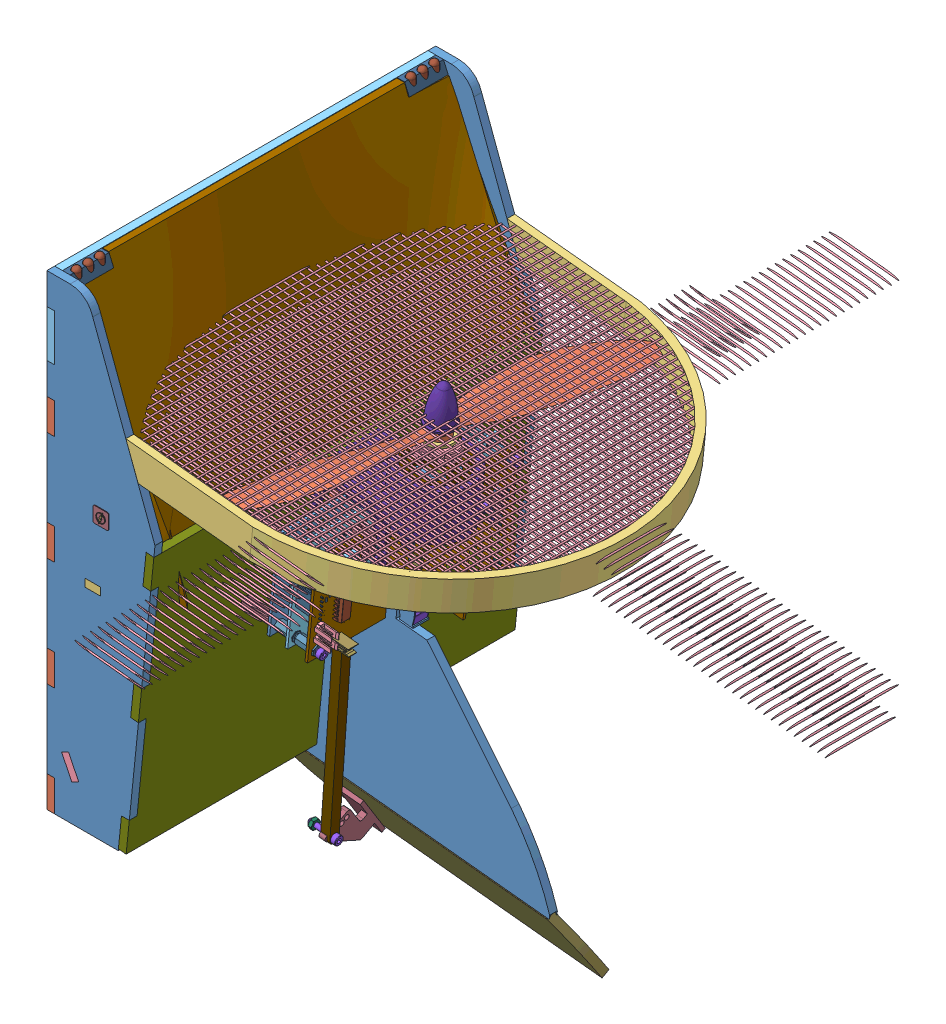
SolidWorks assembly AssTotaleSimu4, configuration Défaut. Lengths in mm. (continued)
Components (placement in the parent): (continued)
- AssStructSimu-1: AssStructSimu [Défaut] at (-125.7658 -1.8483 624.6548) x (1 0 0) z (0 0 -1) size (253.25 324.59 251.6) (continued)
  - AssCarte-1: AssCarte [Défaut] at (38.0121 147.1029 290.772) x (-0.101852 0.9948 0) z (0.9948 0.101852 0) size (66.52 130.57 98.72) (continued)
    - carte_onduleur_v3-1: carte_onduleur_v3 [Défaut] at (-131.8199 12.0892 20.7912) size (66.52 130.57 82.34) (continued)
      - RC2_2-1: RC2_2 [Défaut] at (-22 0.18 -0.803) x (-1 0 0) z (0 0 -1) size (2.34 1.04 0.5) (continued)
        - Open CASCADE STEP translator 6.8 1.12.1-1: Open CASCADE STEP translator 6.8 1.12.1 [Défaut] at origin size (2.34 1.04 0.5) (continued)
          - Pin_2_2-1: Pin_2_2 [Défaut] at origin size (0.51 1.02 0.5)
      - RC3_1-1: RC3_1 [Défaut] at (-20.9336 -14.5 -0.803) x (1 0 0) z (0 0 -1) size (2.34 1.04 0.5)
        - Open CASCADE STEP translator 6.8 1.12.1-1: Open CASCADE STEP translator 6.8 1.12.1 [Défaut] at origin size (2.34 1.04 0.5)
          - Body_1_3-1: Body_1_3 [Défaut] at origin size (2.29 1.04 0.43)
          - Pin_1_2-1: Pin_1_2 [Défaut] at (0.3048 0 0) x (-1 0 0) z (0 0 1) size (0.51 1.02 0.5)
          - Pin_2_2-1: Pin_2_2 [Défaut] at origin size (0.51 1.02 0.5)
      - RC3_2-1: RC3_2 [Défaut] at (-22.3 -14.5 -0.803) x (-1 0 0) z (0 0 -1) size (2.34 1.04 0.5)
        - Open CASCADE STEP translator 6.8 1.12.1-1: Open CASCADE STEP translator 6.8 1.12.1 [Défaut] at origin size (2.34 1.04 0.5)
          - Body_1_3-1: Body_1_3 [Défaut] at origin size (2.29 1.04 0.43)
          - Pin_1_2-1: Pin_1_2 [Défaut] at (0.3048 0 0) x (-1 0 0) z (0 0 1) size (0.51 1.02 0.5)
          - Pin_2_2-1: Pin_2_2 [Défaut] at origin size (0.51 1.02 0.5)
      - U_MES_CUR-1: U_MES_CUR [Défaut] at (-11.5 6.7816 0.803) size (2.54 2.41 0.76)
        - Open CASCADE STEP translator 6.8 1.32.1-1: Open CASCADE STEP translator 6.8 1.32.1 [Défaut] at origin size (2.54 2.41 0.76)
          - Body_1_5-1: Body_1_5 [Défaut] at origin size (2.54 1.27 0.71)
          - Pin_1_3-1: Pin_1_3 [Défaut] at (-2.1082 0.2286 0) x (0 -1 0) z (0 0 1) size (1.14 0.25 0.47)
          - Pin_2_3-1: Pin_2_3 [Défaut] at (-0.2032 2.1336 0) x (0 -1 0) z (0 0 1) size (1.14 0.25 0.47)
      - CARTE_ALIM-1: CARTE_ALIM [Défaut] at (-6.4 -57.2 0.803) size (60 130 18.35)
        - Open CASCADE STEP translator 6.8 1.33.1-1: Open CASCADE STEP translator 6.8 1.33.1 [Défaut] at origin size (60 130 18.35)
          - Body_1_6-1: Body_1_6 [Défaut] at (7 56 -12) size (60 130 18.35)
            - 1_3-1: 1_3 [Défaut] at origin size (60 130 1.61)
            - 13_3-1: 13_3 [Défaut] at (0.4717 -40.93 0.803) x (0 1 0) z (0 0 1) size (5.65 4.9 1.7)
              - =_[0_1_1_4]_3-1: =_[0_1_1_4]_3 [Défaut] at origin size (5.65 4.9 1.7)
                - 2-1: 2 [Défaut] at origin size (3.75 4.9 1.53)
                - 3-1: 3 [Défaut] at origin size (0.95 0.51 1.06)
                - 4-1: 4 [Défaut] at origin size (0.95 0.51 1.06)
                - 5_2-1: 5_2 [Défaut] at origin size (0.95 0.51 1.06)
                - 6-1: 6 [Défaut] at origin size (0.95 0.51 1.06)
                - 7-1: 7 [Défaut] at (10.8 -5.08 0) x (-1 0 0) z (0 0 1) size (0.95 0.51 1.06)
                - 8_2-1: 8_2 [Défaut] at (10.8 -2.54 0) x (-1 0 0) z (0 0 1) size (0.95 0.51 1.06)
                - 9-1: 9 [Défaut] at (10.8 0 0) x (-1 0 0) z (0 0 1) size (0.95 0.51 1.06)
                - 10-1: 10 [Défaut] at (10.8 2.54 0) x (-1 0 0) z (0 0 1) size (0.95 0.51 1.06)
                - 11_2-1: 11_2 [Défaut] at (5.4 -1.27 0) x (-1 0 0) z (0 0 1) size (4.25 2.34 1.06)
            - 18-1: 18 [Défaut] at (-2.5283 -37.23 0.803) x (0 -1 0) z (0 0 1) size (2.34 1.04 0.5)
              - =_[0_1_1_16]-1: =_[0_1_1_16] [Défaut] at origin size (2.34 1.04 0.5)
                - 14_2-1: 14_2 [Défaut] at origin size (2.29 1.04 0.43)
                - 15_2-1: 15_2 [Défaut] at (0.3048 0 0) x (-1 0 0) z (0 0 1) size (0.51 1.02 0.5)
                - 16_2-1: 16_2 [Défaut] at origin size (0.51 1.02 0.5)
            - 21_2-1: 21_2 [Défaut] at (-2.2263 -24.628 -0.803) x (1 0 0) z (0 0 -1) size (8.01 8 14.24)
              - =_[0_1_1_21]-1: =_[0_1_1_21] [Défaut] at origin size (8.01 8 14.24)
                - 19-1: 19 [Défaut] at (1.8 0 0) x (1 0 0) z (0 -1 0) size (8.01 14.24 8)
            - 23_2-1: 23_2 [Défaut] at (1.2381 -31.53 0.803) size (2.34 1.04 0.5)
              - =_[0_1_1_16]-1: =_[0_1_1_16] [Défaut] at origin size (2.34 1.04 0.5)
                - 14_2-1: 14_2 [Défaut] at origin size (2.29 1.04 0.43)
                - 15_2-1: 15_2 [Défaut] at (0.3048 0 0) x (-1 0 0) z (0 0 1) size (0.51 1.02 0.5)
                - 16_2-1: 16_2 [Défaut] at origin size (0.51 1.02 0.5)
            - 28-1: 28 [Défaut] at (5 29.8636 0.803) x (0 -1 0) z (0 0 1) size (3.35 1.3 0.55)
              - =_[0_1_1_25]_2-1: =_[0_1_1_25]_2 [Défaut] at origin size (3.35 1.3 0.55)
                - 24-1: 24 [Défaut] at origin size (3.3 1.3 0.48)
                - 25_2-1: 25_2 [Défaut] at (0.5588 0 0) x (-1 0 0) z (0 0 1) size (0.76 1.27 0.55)
                - 26_2-1: 26_2 [Défaut] at origin size (0.76 1.27 0.55)
            - 30-1: 30 [Défaut] at (6.7 29.8636 0.803) x (0 -1 0) z (0 0 1) size (2.34 1.04 0.5)
              - =_[0_1_1_16]-1: =_[0_1_1_16] [Défaut] at origin size (2.34 1.04 0.5)
                - 14_2-1: 14_2 [Défaut] at origin size (2.29 1.04 0.43)
                - 15_2-1: 15_2 [Défaut] at (0.3048 0 0) x (-1 0 0) z (0 0 1) size (0.51 1.02 0.5)
                - 16_2-1: 16_2 [Défaut] at origin size (0.51 1.02 0.5)
            - 35_2-1: 35_2 [Défaut] at (-2.5 -46.37 0.803) x (0 1 0) z (0 0 1) size (3.4 2.06 0.79)
              - =_[0_1_1_31]-1: =_[0_1_1_31] [Défaut] at origin size (3.4 2.06 0.79)
                - 31_2-1: 31_2 [Défaut] at origin size (3.3 2.06 0.69)
                - 32_3-1: 32_3 [Défaut] at (0.5588 0 0) x (-1 0 0) z (0 0 1) size (0.81 2.03 0.79)
                - 33_3-1: 33_3 [Défaut] at origin size (0.81 2.03 0.79)
            - 37-1: 37 [Défaut] at (5 31.43 0.803) x (0 1 0) z (0 0 1) size (2.34 1.04 0.5)
              - =_[0_1_1_16]-1: =_[0_1_1_16] [Défaut] at origin size (2.34 1.04 0.5)
                - 14_2-1: 14_2 [Défaut] at origin size (2.29 1.04 0.43)
                - 15_2-1: 15_2 [Défaut] at (0.3048 0 0) x (-1 0 0) z (0 0 1) size (0.51 1.02 0.5)
                - 16_2-1: 16_2 [Défaut] at origin size (0.51 1.02 0.5)
            - 39-1: 39 [Défaut] at (-0.2 35.63 0.803) x (-1 0 0) z (0 0 1) size (2.34 1.04 0.5)
              - =_[0_1_1_16]-1: =_[0_1_1_16] [Défaut] at origin size (2.34 1.04 0.5)
                - 14_2-1: 14_2 [Défaut] at origin size (2.29 1.04 0.43)
                - 15_2-1: 15_2 [Défaut] at (0.3048 0 0) x (-1 0 0) z (0 0 1) size (0.51 1.02 0.5)
                - 16_2-1: 16_2 [Défaut] at origin size (0.51 1.02 0.5)
            - 41-1: 41 [Défaut] at (2.9 -45.5036 0.803) x (0 1 0) z (0 0 1) size (2.34 1.04 0.5)
              - =_[0_1_1_16]-1: =_[0_1_1_16] [Défaut] at origin size (2.34 1.04 0.5)
                - 14_2-1: 14_2 [Défaut] at origin size (2.29 1.04 0.43)
                - 15_2-1: 15_2 [Défaut] at (0.3048 0 0) x (-1 0 0) z (0 0 1) size (0.51 1.02 0.5)
                - 16_2-1: 16_2 [Défaut] at origin size (0.51 1.02 0.5)
            - 43-1: 43 [Défaut] at (17.1348 -42.6272 0.803) x (0 1 0) z (0 0 1) size (2.34 1.04 0.5)
              - =_[0_1_1_16]-1: =_[0_1_1_16] [Défaut] at origin size (2.34 1.04 0.5)
                - 14_2-1: 14_2 [Défaut] at origin size (2.29 1.04 0.43)
                - 15_2-1: 15_2 [Défaut] at (0.3048 0 0) x (-1 0 0) z (0 0 1) size (0.51 1.02 0.5)
                - 16_2-1: 16_2 [Défaut] at origin size (0.51 1.02 0.5)
            - 48_2-1: 48_2 [Défaut] at (-5.4717 -39.01 0.803) x (-1 0 0) z (0 0 1) size (4.19 3.4 1.75)
              - =_[0_1_1_40]-1: =_[0_1_1_40] [Défaut] at origin size (4.19 3.4 1.75)
                - 44_2-1: 44_2 [Défaut] at origin size (3.75 3.38 1.73)
                - 45_2-1: 45_2 [Défaut] at (0.438 0 0) x (-1 0 0) z (0 0 1) size (0.53 3.4 1.75)
                - 46_2-1: 46_2 [Défaut] at origin size (0.52 3.4 1.75)
            - 53-1: 53 [Défaut] at (0.9 35.63 0.803) size (2.34 1.04 0.5)
              - =_[0_1_1_45]-1: =_[0_1_1_45] [Défaut] at origin size (2.34 1.04 0.5)
                - 49_3-1: 49_3 [Défaut] at origin size (2.29 1.04 0.43)
                - 50-1: 50 [Défaut] at (0.3048 0 0) x (-1 0 0) z (0 0 1) size (0.51 1.02 0.5)
                - 51-1: 51 [Défaut] at origin size (0.51 1.02 0.5)
            - 55_2-1: 55_2 [Défaut] at (1.3 -45.5036 0.803) x (0 1 0) z (0 0 1) size (2.34 1.04 0.5)
              - =_[0_1_1_45]-1: =_[0_1_1_45] [Défaut] at origin size (2.34 1.04 0.5)
                - 49_3-1: 49_3 [Défaut] at origin size (2.29 1.04 0.43)
                - 50-1: 50 [Défaut] at (0.3048 0 0) x (-1 0 0) z (0 0 1) size (0.51 1.02 0.5)
                - 51-1: 51 [Défaut] at origin size (0.51 1.02 0.5)
            - 57_3-1: 57_3 [Défaut] at (17.2348 -43.9936 0.803) x (0 -1 0) z (0 0 1) size (2.34 1.04 0.5)
              - =_[0_1_1_45]-1: =_[0_1_1_45] [Défaut] at origin size (2.34 1.04 0.5)
                - 49_3-1: 49_3 [Défaut] at origin size (2.29 1.04 0.43)
                - 50-1: 50 [Défaut] at (0.3048 0 0) x (-1 0 0) z (0 0 1) size (0.51 1.02 0.5)
                - 51-1: 51 [Défaut] at origin size (0.51 1.02 0.5)
            - 65-1: 65 [Défaut] at (-4.8 30.93 0.803) x (-1 0 0) z (0 0 1) size (14.64 9.83 4.25)
              - =_[0_1_1_52]-1: =_[0_1_1_52] [Défaut] at origin size (14.64 9.83 4.25)
                - 63_2-1: 63_2 [Défaut] at (3 0 0) x (0 -1 0) z (0 0 1) size (9.83 14.64 4.25)
                  - =_[0_1_1_3]_5-1: =_[0_1_1_3]_5 [Défaut] at origin size (9.83 9.05 4.21)
                  - =_[0_1_1_4]_5-1: =_[0_1_1_4]_5 [Défaut] at origin size (9.48 7.76 1.21)
                  - =_[0_1_1_5]_5-1: =_[0_1_1_5]_5 [Défaut] at origin size (1.36 6.01 3.08)
                  - =_[0_1_1_6]_3-1: =_[0_1_1_6]_3 [Défaut] at origin size (1.36 6.01 3.08)
                  - =_[0_1_1_7]_3-1: =_[0_1_1_7]_3 [Défaut] at origin size (1.06 6.01 3.08)
            - 67-1: 67 [Défaut] at (13.5933 -37.5272 0.803) x (-1 0 0) z (0 0 1) size (2.34 1.04 0.5)
              - =_[0_1_1_16]-1: =_[0_1_1_16] [Défaut] at origin size (2.34 1.04 0.5)
                - 14_2-1: 14_2 [Défaut] at origin size (2.29 1.04 0.43)
                - 15_2-1: 15_2 [Défaut] at (0.3048 0 0) x (-1 0 0) z (0 0 1) size (0.51 1.02 0.5)
                - 16_2-1: 16_2 [Défaut] at origin size (0.51 1.02 0.5)
            - 70_2-1: 70_2 [Défaut] at (18.2733 -29.7272 0.803) x (0 1 0) z (0 0 1) size (6.06 4.95 1.88)
              - =_[0_1_1_61]-1: =_[0_1_1_61] [Défaut] at origin size (6.06 4.95 1.88)
                - 68-1: 68 [Défaut] x (1 0 0) z (0 -1 0) size (6.06 1.88 4.95)
            - 83-1: 83 [Défaut] at (-21.2 -38.07 0.803) x (-1 0 0) z (0 0 1) size (2.7 5.2 1.11)
              - =_[0_1_1_64]-1: =_[0_1_1_64] [Défaut] at origin size (2.7 5.2 1.11)
                - 84_2-1: 84_2 [Défaut] at (1.2 -4 0) x (0 1 0) z (0 0 1) size (5.2 2.7 1.11)
                  - =_[0_1_1_3]_6-1: =_[0_1_1_3]_6 [Défaut] at origin size (0.39 0.64 0.01)
                  - =_[0_1_1_4]_6-1: =_[0_1_1_4]_6 [Défaut] at origin size (0.6 1.9 0.2)
                  - =_[0_1_1_5]_6-1: =_[0_1_1_5]_6 [Défaut] at origin size (0.21 0.08 0.01)
                  - =_[0_1_1_6]_4-1: =_[0_1_1_6]_4 [Défaut] at origin size (0.6 1.9 0.2)
                  - =_[0_1_1_7]_4-1: =_[0_1_1_7]_4 [Défaut] at origin size (0.46 0.68 0.01)
                  - =_[0_1_1_8]_3-1: =_[0_1_1_8]_3 [Défaut] at origin size (0.38 0.66 0.01)
                  - =_[0_1_1_9]_2-1: =_[0_1_1_9]_2 [Défaut] at origin size (0.2 0.62 0.01)
                  - =_[0_1_1_10]_2-1: =_[0_1_1_10]_2 [Défaut] at origin size (4 2.7 1.1)
                  - =_[0_1_1_11]_2-1: =_[0_1_1_11]_2 [Défaut] at origin size (0.46 0.63 0.01)
                  - =_[0_1_1_12]_2-1: =_[0_1_1_12]_2 [Défaut] at origin size (0.56 0.68 0.01)
            - 86_2-1: 86_2 [Défaut] at (12.8933 -35.4272 0.803) x (0 1 0) z (0 0 1) size (2.7 5.2 1.11)
              - =_[0_1_1_77]-1: =_[0_1_1_77] [Défaut] at origin size (2.7 5.2 1.11)
                - 84_2-1: 84_2 [Défaut] at (1.2 -4 0) x (0 1 0) z (0 0 1) size (5.2 2.7 1.11)
                  - =_[0_1_1_3]_6-1: =_[0_1_1_3]_6 [Défaut] at origin size (0.39 0.64 0.01)
                  - =_[0_1_1_4]_6-1: =_[0_1_1_4]_6 [Défaut] at origin size (0.6 1.9 0.2)
                  - =_[0_1_1_5]_6-1: =_[0_1_1_5]_6 [Défaut] at origin size (0.21 0.08 0.01)
                  - =_[0_1_1_6]_4-1: =_[0_1_1_6]_4 [Défaut] at origin size (0.6 1.9 0.2)
                  - =_[0_1_1_7]_4-1: =_[0_1_1_7]_4 [Défaut] at origin size (0.46 0.68 0.01)
                  - =_[0_1_1_8]_3-1: =_[0_1_1_8]_3 [Défaut] at origin size (0.38 0.66 0.01)
                  - =_[0_1_1_9]_2-1: =_[0_1_1_9]_2 [Défaut] at origin size (0.2 0.62 0.01)
                  - =_[0_1_1_10]_2-1: =_[0_1_1_10]_2 [Défaut] at origin size (4 2.7 1.1)
                  - =_[0_1_1_11]_2-1: =_[0_1_1_11]_2 [Défaut] at origin size (0.46 0.63 0.01)
                  - =_[0_1_1_12]_2-1: =_[0_1_1_12]_2 [Défaut] at origin size (0.56 0.68 0.01)
            - 92_2-1: 92_2 [Défaut] at (20.9933 -39.3272 0.803) x (0 -1 0) z (0 0 1) size (2.79 1.98 0.64)
              - =_[0_1_1_79]-1: =_[0_1_1_79] [Défaut] at origin size (2.79 1.98 0.64)
                - 87-1: 87 [Défaut] at origin size (2.79 1.02 0.58)
                - 88-1: 88 [Défaut] x (0 -1 0) z (0 0 1) size (0.42 0.38 0.38)
                - 89-1: 89 [Défaut] at (-2.8448 -0.9652 0) x (0 1 0) z (0 0 1) size (0.55 0.38 0.38)
                - 90-1: 90 [Défaut] at (-0.9652 -2.8448 0) x (0 1 0) z (0 0 1) size (0.55 0.38 0.38)
            - 98-1: 98 [Défaut] at (-17.7 -48.47 0.803) x (0 -1 0) z (0 0 1) size (2.54 1.98 0.64)
              - =_[0_1_1_85]-1: =_[0_1_1_85] [Défaut] at origin size (2.54 1.98 0.64)
                - 93-1: 93 [Défaut] at origin size (2.54 1.14 0.58)
                - 94-1: 94 [Défaut] x (0 -1 0) z (0 0 1) size (0.43 0.51 0.38)
                - 95-1: 95 [Défaut] at (1.8796 1.8796 0) x (0 -1 0) z (0 0 1) size (0.43 0.51 0.38)
                - 96-1: 96 [Défaut] at (-0.9652 -2.8448 0) x (0 1 0) z (0 0 1) size (0.41 0.51 0.38)
            - 100-1: 100 [Défaut] at (24.3933 -43.2272 0.803) size (2.79 1.98 0.64)
              - =_[0_1_1_79]-1: =_[0_1_1_79] [Défaut] at origin size (2.79 1.98 0.64)
                - 87-1: 87 [Défaut] at origin size (2.79 1.02 0.58)
                - 88-1: 88 [Défaut] x (0 -1 0) z (0 0 1) size (0.42 0.38 0.38)
                - 89-1: 89 [Défaut] at (-2.8448 -0.9652 0) x (0 1 0) z (0 0 1) size (0.55 0.38 0.38)
                - 90-1: 90 [Défaut] at (-0.9652 -2.8448 0) x (0 1 0) z (0 0 1) size (0.55 0.38 0.38)
            - 102-1: 102 [Défaut] at (21.4933 -44.4272 0.803) x (0 -1 0) z (0 0 1) size (2.79 1.98 0.64)
              - =_[0_1_1_79]-1: =_[0_1_1_79] [Défaut] at origin size (2.79 1.98 0.64)
                - 87-1: 87 [Défaut] at origin size (2.79 1.02 0.58)
                - 88-1: 88 [Défaut] x (0 -1 0) z (0 0 1) size (0.42 0.38 0.38)
                - 89-1: 89 [Défaut] at (-2.8448 -0.9652 0) x (0 1 0) z (0 0 1) size (0.55 0.38 0.38)
                - 90-1: 90 [Défaut] at (-0.9652 -2.8448 0) x (0 1 0) z (0 0 1) size (0.55 0.38 0.38)
            - 107-1: 107 [Défaut] at (23.1933 -29.1272 -0.803) x (0 1 0) z (0 0 -1) size (9.6 14.35 5)
              - =_[0_1_1_93]-1: =_[0_1_1_93] [Défaut] at origin size (9.6 14.35 5)
                - 105-1: 105 [Défaut] at (0.5 -1 2) x (-1 0 0) z (0 0 1) size (9.6 14.35 5)
                  - =_[0_1_1_3]_7-1: =_[0_1_1_3]_7 [Défaut] at origin size (9.6 12.75 5)
                  - =_[0_1_1_4]_7-1: =_[0_1_1_4]_7 [Défaut] at origin size (2.2 1.6 2.2)
            - 109-1: 109 [Défaut] at (25.4933 -41.1272 0.803) x (-1 0 0) z (0 0 1) size (2.34 1.04 0.5)
              - =_[0_1_1_45]-1: =_[0_1_1_45] [Défaut] at origin size (2.34 1.04 0.5)
                - 49_3-1: 49_3 [Défaut] at origin size (2.29 1.04 0.43)
                - 50-1: 50 [Défaut] at (0.3048 0 0) x (-1 0 0) z (0 0 1) size (0.51 1.02 0.5)
                - 51-1: 51 [Défaut] at origin size (0.51 1.02 0.5)
            - 111-1: 111 [Défaut] at (22.0269 -41.8272 0.803) x (-1 0 0) z (0 0 1) size (2.34 1.04 0.5)
              - =_[0_1_1_45]-1: =_[0_1_1_45] [Défaut] at origin size (2.34 1.04 0.5)
                - 49_3-1: 49_3 [Défaut] at origin size (2.29 1.04 0.43)
                - 50-1: 50 [Défaut] at (0.3048 0 0) x (-1 0 0) z (0 0 1) size (0.51 1.02 0.5)
                - 51-1: 51 [Défaut] at origin size (0.51 1.02 0.5)
            - 113-1: 113 [Défaut] at (-24.8 -36.7036 0.803) x (0 1 0) z (0 0 1) size (2.34 1.04 0.5)
              - =_[0_1_1_45]-1: =_[0_1_1_45] [Défaut] at origin size (2.34 1.04 0.5)
                - 49_3-1: 49_3 [Défaut] at origin size (2.29 1.04 0.43)
                - 50-1: 50 [Défaut] at (0.3048 0 0) x (-1 0 0) z (0 0 1) size (0.51 1.02 0.5)
                - 51-1: 51 [Défaut] at origin size (0.51 1.02 0.5)
            - 115-1: 115 [Défaut] at (-24.8 -40.3036 0.803) x (0 1 0) z (0 0 1) size (2.34 1.04 0.5)
              - =_[0_1_1_45]-1: =_[0_1_1_45] [Défaut] at origin size (2.34 1.04 0.5)
                - 49_3-1: 49_3 [Défaut] at origin size (2.29 1.04 0.43)
                - 50-1: 50 [Défaut] at (0.3048 0 0) x (-1 0 0) z (0 0 1) size (0.51 1.02 0.5)
                - 51-1: 51 [Défaut] at origin size (0.51 1.02 0.5)
            - 117-1: 117 [Défaut] at (-16 -48.27 0.803) x (0 -1 0) z (0 0 1) size (2.34 1.04 0.5)
              - =_[0_1_1_45]-1: =_[0_1_1_45] [Défaut] at origin size (2.34 1.04 0.5)
                - 49_3-1: 49_3 [Défaut] at origin size (2.29 1.04 0.43)
                - 50-1: 50 [Défaut] at (0.3048 0 0) x (-1 0 0) z (0 0 1) size (0.51 1.02 0.5)
                - 51-1: 51 [Défaut] at origin size (0.51 1.02 0.5)
            - 119-1: 119 [Défaut] at (-22.5189 -47.87 0.803) x (-1 0 0) z (0 0 1) size (2.34 1.04 0.5)
              - =_[0_1_1_45]-1: =_[0_1_1_45] [Défaut] at origin size (2.34 1.04 0.5)
                - 49_3-1: 49_3 [Défaut] at origin size (2.29 1.04 0.43)
                - 50-1: 50 [Défaut] at (0.3048 0 0) x (-1 0 0) z (0 0 1) size (0.51 1.02 0.5)
                - 51-1: 51 [Défaut] at origin size (0.51 1.02 0.5)
            - 121-1: 121 [Défaut] at (22.3933 -38.9272 0.803) size (2.34 1.04 0.5)
              - =_[0_1_1_45]-1: =_[0_1_1_45] [Défaut] at origin size (2.34 1.04 0.5)
                - 49_3-1: 49_3 [Défaut] at origin size (2.29 1.04 0.43)
                - 50-1: 50 [Défaut] at (0.3048 0 0) x (-1 0 0) z (0 0 1) size (0.51 1.02 0.5)
                - 51-1: 51 [Défaut] at origin size (0.51 1.02 0.5)
            - 123-1: 123 [Défaut] at (22.0933 -36.4272 0.803) x (-1 0 0) z (0 0 1) size (2.34 1.04 0.5)
              - =_[0_1_1_45]-1: =_[0_1_1_45] [Défaut] at origin size (2.34 1.04 0.5)
                - 49_3-1: 49_3 [Défaut] at origin size (2.29 1.04 0.43)
                - 50-1: 50 [Défaut] at (0.3048 0 0) x (-1 0 0) z (0 0 1) size (0.51 1.02 0.5)
                - 51-1: 51 [Défaut] at origin size (0.51 1.02 0.5)
            - 125-1: 125 [Défaut] at (22.3933 -32.0272 0.803) x (0 -1 0) z (0 0 1) size (2.34 1.04 0.5)
              - =_[0_1_1_45]-1: =_[0_1_1_45] [Défaut] at origin size (2.34 1.04 0.5)
                - 49_3-1: 49_3 [Défaut] at origin size (2.29 1.04 0.43)
                - 50-1: 50 [Défaut] at (0.3048 0 0) x (-1 0 0) z (0 0 1) size (0.51 1.02 0.5)
                - 51-1: 51 [Défaut] at origin size (0.51 1.02 0.5)
            - 127-1: 127 [Défaut] at (17.9597 -23.1272 0.803) size (2.34 1.04 0.5)
              - =_[0_1_1_16]-1: =_[0_1_1_16] [Défaut] at origin size (2.34 1.04 0.5)
                - 14_2-1: 14_2 [Défaut] at origin size (2.29 1.04 0.43)
                - 15_2-1: 15_2 [Défaut] at (0.3048 0 0) x (-1 0 0) z (0 0 1) size (0.51 1.02 0.5)
                - 16_2-1: 16_2 [Défaut] at origin size (0.51 1.02 0.5)
            - 129-1: 129 [Défaut] at (20.0269 -24.9272 0.803) x (-1 0 0) z (0 0 1) size (2.34 1.04 0.5)
              - =_[0_1_1_16]-1: =_[0_1_1_16] [Défaut] at origin size (2.34 1.04 0.5)
                - 14_2-1: 14_2 [Défaut] at origin size (2.29 1.04 0.43)
                - 15_2-1: 15_2 [Défaut] at (0.3048 0 0) x (-1 0 0) z (0 0 1) size (0.51 1.02 0.5)
                - 16_2-1: 16_2 [Défaut] at origin size (0.51 1.02 0.5)
            - 131-1: 131 [Défaut] at (16.9933 -37.5272 0.803) x (-1 0 0) z (0 0 1) size (2.34 1.04 0.5)
              - =_[0_1_1_45]-1: =_[0_1_1_45] [Défaut] at origin size (2.34 1.04 0.5)
                - 49_3-1: 49_3 [Défaut] at origin size (2.29 1.04 0.43)
                - 50-1: 50 [Défaut] at (0.3048 0 0) x (-1 0 0) z (0 0 1) size (0.51 1.02 0.5)
                - 51-1: 51 [Défaut] at origin size (0.51 1.02 0.5)
            - 136-1: 136 [Défaut] at (3.2957 -29.23 0.803) x (-1 0 0) z (0 0 1) size (4.78 2.79 2.03)
              - =_[0_1_1_110]_2-1: =_[0_1_1_110]_2 [Défaut] at origin size (4.78 2.79 2.03)
                - 132-1: 132 [Défaut] at origin size (4.32 2.79 1.78)
                - 133-1: 133 [Défaut] at (0.4572 0 0) x (-1 0 0) z (0 0 1) size (1.02 1.27 1.32)
                - 134-1: 134 [Défaut] at origin size (1.02 1.27 1.32)
            - 141-1: 141 [Défaut] at (0.2436 -33.3673 0.803) size (3.35 1.3 0.55)
              - =_[0_1_1_115]_2-1: =_[0_1_1_115]_2 [Défaut] at origin size (3.35 1.3 0.55)
                - 137-1: 137 [Défaut] at origin size (3.3 1.3 0.48)
                - 138-1: 138 [Défaut] at (0.5588 0 0) x (-1 0 0) z (0 0 1) size (0.76 1.27 0.55)
                - 139-1: 139 [Défaut] at origin size (0.76 1.27 0.55)
            - 143_2-1: 143_2 [Défaut] at (-0.3 -45.47 0.803) x (0 1 0) z (0 0 1) size (2.34 1.04 0.5)
              - =_[0_1_1_16]-1: =_[0_1_1_16] [Défaut] at origin size (2.34 1.04 0.5)
                - 14_2-1: 14_2 [Défaut] at origin size (2.29 1.04 0.43)
                - 15_2-1: 15_2 [Défaut] at (0.3048 0 0) x (-1 0 0) z (0 0 1) size (0.51 1.02 0.5)
                - 16_2-1: 16_2 [Défaut] at origin size (0.51 1.02 0.5)
            - 145-1: 145 [Défaut] at (6.6 31.13 0.803) x (0 1 0) z (0 0 1) size (3.35 1.3 0.55)
              - =_[0_1_1_25]_2-1: =_[0_1_1_25]_2 [Défaut] at origin size (3.35 1.3 0.55)
                - 24-1: 24 [Défaut] at origin size (3.3 1.3 0.48)
                - 25_2-1: 25_2 [Défaut] at (0.5588 0 0) x (-1 0 0) z (0 0 1) size (0.76 1.27 0.55)
                - 26_2-1: 26_2 [Défaut] at origin size (0.76 1.27 0.55)
            - 148-1: 148 [Défaut] at (-7.5 -56.57 0.803) size (15.24 2.54 7.37)
              - =_[0_1_1_122]_2-1: =_[0_1_1_122]_2 [Défaut] at origin size (15.24 2.54 7.37)
                - 146-1: 146 [Défaut] at (6.3 0 1) x (1 0 0) z (0 -1 0) size (15.24 7.37 2.54)
      - COMP1-1: COMP1 [Défaut] at (-16.3 -36.2 0.803) x (-1 0 0) z (0 0 1) size (2.03 1.88 0.51)
        - Open CASCADE STEP translator 6.8 1.34.1-1: Open CASCADE STEP translator 6.8 1.34.1 [Défaut] at origin size (2.03 1.88 0.51)
          - Body_1_6-1: Body_1_6 [Défaut] at origin size (2.03 1.02 0.46)
          - Pin_1_4-1: Pin_1_4 [Défaut] x (0 1 0) z (0 0 1) size (0.45 0.25 0.32)
          - Pin_2_4-1: Pin_2_4 [Défaut] at (0.65 -0.65 0) x (0 1 0) z (0 0 1) size (0.45 0.25 0.32)
          - Pin_3-1: Pin_3 [Défaut] at (1.3 -1.3 0) x (0 1 0) z (0 0 1) size (0.45 0.25 0.32)
          - Pin_4-1: Pin_4 [Défaut] at (-0.5 3.1 0) x (0 -1 0) z (0 0 1) size (0.41 0.25 0.32)
          - Pin_5-1: Pin_5 [Défaut] at (-1.8 1.8 0) x (0 -1 0) z (0 0 1) size (0.41 0.25 0.32)
      - COMP2-1: COMP2 [Défaut] at (-14.3 -9.6 0.803) x (-1 0 0) z (0 0 1) size (2.03 1.88 0.51)
        - Open CASCADE STEP translator 6.8 1.34.1-1: Open CASCADE STEP translator 6.8 1.34.1 [Défaut] at origin size (2.03 1.88 0.51)
          - Body_1_6-1: Body_1_6 [Défaut] at origin size (2.03 1.02 0.46)
          - Pin_1_4-1: Pin_1_4 [Défaut] x (0 1 0) z (0 0 1) size (0.45 0.25 0.32)
          - Pin_2_4-1: Pin_2_4 [Défaut] at (0.65 -0.65 0) x (0 1 0) z (0 0 1) size (0.45 0.25 0.32)
          - Pin_3-1: Pin_3 [Défaut] at (1.3 -1.3 0) x (0 1 0) z (0 0 1) size (0.45 0.25 0.32)
          - Pin_4-1: Pin_4 [Défaut] at (-0.5 3.1 0) x (0 -1 0) z (0 0 1) size (0.41 0.25 0.32)
          - Pin_5-1: Pin_5 [Défaut] at (-1.8 1.8 0) x (0 -1 0) z (0 0 1) size (0.41 0.25 0.32)
      - COMP3-1: COMP3 [Défaut] at (-15.9 -23.2 0.803) x (-1 0 0) z (0 0 1) size (2.03 1.88 0.51)
        - Open CASCADE STEP translator 6.8 1.34.1-1: Open CASCADE STEP translator 6.8 1.34.1 [Défaut] at origin size (2.03 1.88 0.51)
          - Body_1_6-1: Body_1_6 [Défaut] at origin size (2.03 1.02 0.46)
          - Pin_1_4-1: Pin_1_4 [Défaut] x (0 1 0) z (0 0 1) size (0.45 0.25 0.32)
          - Pin_2_4-1: Pin_2_4 [Défaut] at (0.65 -0.65 0) x (0 1 0) z (0 0 1) size (0.45 0.25 0.32)
          - Pin_3-1: Pin_3 [Défaut] at (1.3 -1.3 0) x (0 1 0) z (0 0 1) size (0.45 0.25 0.32)
          - Pin_4-1: Pin_4 [Défaut] at (-0.5 3.1 0) x (0 -1 0) z (0 0 1) size (0.41 0.25 0.32)
          - Pin_5-1: Pin_5 [Défaut] at (-1.8 1.8 0) x (0 -1 0) z (0 0 1) size (0.41 0.25 0.32)
      - CP1-1: CP1 [Défaut] at (-18.9 -38.2 0.803) x (0 1 0) z (0 0 1) size (2.34 1.04 0.5)
        - Open CASCADE STEP translator 6.8 1.6.1-1: Open CASCADE STEP translator 6.8 1.6.1 [Défaut] at origin size (2.34 1.04 0.5)
          - Body_1-1: Body_1 [Défaut] at origin size (2.29 1.04 0.43)
          - Pin_1-1: Pin_1 [Défaut] at (0.3048 0 0) x (-1 0 0) z (0 0 1) size (0.51 1.02 0.5)
          - Pin_2-1: Pin_2 [Défaut] at origin size (0.51 1.02 0.5)
      - CP2-1: CP2 [Défaut] at (-16.9 -11.6 0.803) x (0 1 0) z (0 0 1) size (2.34 1.04 0.5)
        - Open CASCADE STEP translator 6.8 1.6.1-1: Open CASCADE STEP translator 6.8 1.6.1 [Défaut] at origin size (2.34 1.04 0.5)
          - Body_1-1: Body_1 [Défaut] at origin size (2.29 1.04 0.43)
          - Pin_1-1: Pin_1 [Défaut] at (0.3048 0 0) x (-1 0 0) z (0 0 1) size (0.51 1.02 0.5)
          - Pin_2-1: Pin_2 [Défaut] at origin size (0.51 1.02 0.5)
      - CP3-1: CP3 [Défaut] at (-18.5 -25.2 0.803) x (0 1 0) z (0 0 1) size (2.34 1.04 0.5)
        - Open CASCADE STEP translator 6.8 1.6.1-1: Open CASCADE STEP translator 6.8 1.6.1 [Défaut] at origin size (2.34 1.04 0.5)
          - Body_1-1: Body_1 [Défaut] at origin size (2.29 1.04 0.43)
          - Pin_1-1: Pin_1 [Défaut] at (0.3048 0 0) x (-1 0 0) z (0 0 1) size (0.51 1.02 0.5)
          - Pin_2-1: Pin_2 [Défaut] at origin size (0.51 1.02 0.5)
      - C_DEC_COM1-1: C_DEC_COM1 [Défaut] at (-15 -36 0.803) x (0 -1 0) z (0 0 1) size (2.34 1.04 0.5)
        - Open CASCADE STEP translator 6.8 1.6.1-1: Open CASCADE STEP translator 6.8 1.6.1 [Défaut] at origin size (2.34 1.04 0.5)
          - Body_1-1: Body_1 [Défaut] at origin size (2.29 1.04 0.43)
          - Pin_1-1: Pin_1 [Défaut] at (0.3048 0 0) x (-1 0 0) z (0 0 1) size (0.51 1.02 0.5)
          - Pin_2-1: Pin_2 [Défaut] at origin size (0.51 1.02 0.5)
      - C_DEC_COMP2-1: C_DEC_COMP2 [Défaut] at (-13 -9.3 0.803) x (0 -1 0) z (0 0 1) size (2.34 1.04 0.5)
        - Open CASCADE STEP translator 6.8 1.6.1-1: Open CASCADE STEP translator 6.8 1.6.1 [Défaut] at origin size (2.34 1.04 0.5)
          - Body_1-1: Body_1 [Défaut] at origin size (2.29 1.04 0.43)
          - Pin_1-1: Pin_1 [Défaut] at (0.3048 0 0) x (-1 0 0) z (0 0 1) size (0.51 1.02 0.5)
          - Pin_2-1: Pin_2 [Défaut] at origin size (0.51 1.02 0.5)
      - C_DEC_COMP3-1: C_DEC_COMP3 [Défaut] at (-14.6 -22.9 0.803) x (0 -1 0) z (0 0 1) size (2.34 1.04 0.5)
        - Open CASCADE STEP translator 6.8 1.6.1-1: Open CASCADE STEP translator 6.8 1.6.1 [Défaut] at origin size (2.34 1.04 0.5)
          - Body_1-1: Body_1 [Défaut] at origin size (2.29 1.04 0.43)
          - Pin_1-1: Pin_1 [Défaut] at (0.3048 0 0) x (-1 0 0) z (0 0 1) size (0.51 1.02 0.5)
          - Pin_2-1: Pin_2 [Défaut] at origin size (0.51 1.02 0.5)
      - D_VBAT-1: D_VBAT [Défaut] at (-1.2 46.4 0.803) x (0 -1 0) z (0 0 1) size (2.34 1.04 0.5)
        - Open CASCADE STEP translator 6.8 1.6.1-1: Open CASCADE STEP translator 6.8 1.6.1 [Défaut] at origin size (2.34 1.04 0.5)
          - Body_1-1: Body_1 [Défaut] at origin size (2.29 1.04 0.43)
          - Pin_1-1: Pin_1 [Défaut] at (0.3048 0 0) x (-1 0 0) z (0 0 1) size (0.51 1.02 0.5)
          - Pin_2-1: Pin_2 [Défaut] at origin size (0.51 1.02 0.5)
      - D_3V-1: D_3V [Défaut] at (1.3 46.3 0.803) x (0 -1 0) z (0 0 1) size (2.34 1.04 0.5)
        - Open CASCADE STEP translator 6.8 1.6.1-1: Open CASCADE STEP translator 6.8 1.6.1 [Défaut] at origin size (2.34 1.04 0.5)
          - Body_1-1: Body_1 [Défaut] at origin size (2.29 1.04 0.43)
          - Pin_1-1: Pin_1 [Défaut] at (0.3048 0 0) x (-1 0 0) z (0 0 1) size (0.51 1.02 0.5)
          - Pin_2-1: Pin_2 [Défaut] at origin size (0.51 1.02 0.5)
      - D_5V-1: D_5V [Défaut] at (-3.7 46.4 0.803) x (0 -1 0) z (0 0 1) size (2.34 1.04 0.5)
        - Open CASCADE STEP translator 6.8 1.6.1-1: Open CASCADE STEP translator 6.8 1.6.1 [Défaut] at origin size (2.34 1.04 0.5)
          - Body_1-1: Body_1 [Défaut] at origin size (2.29 1.04 0.43)
          - Pin_1-1: Pin_1 [Défaut] at (0.3048 0 0) x (-1 0 0) z (0 0 1) size (0.51 1.02 0.5)
          - Pin_2-1: Pin_2 [Défaut] at origin size (0.51 1.02 0.5)
      - R1_1-1: R1_1 [Défaut] at (-20.2 -36.1 0.803) x (-1 0 0) z (0 0 1) size (2.34 1.04 0.5)
        - Open CASCADE STEP translator 6.8 1.12.1-1: Open CASCADE STEP translator 6.8 1.12.1 [Défaut] at origin size (2.34 1.04 0.5)
          - Body_1_3-1: Body_1_3 [Défaut] at origin size (2.29 1.04 0.43)
          - Pin_1_2-1: Pin_1_2 [Défaut] at (0.3048 0 0) x (-1 0 0) z (0 0 1) size (0.51 1.02 0.5)
          - Pin_2_2-1: Pin_2_2 [Défaut] at origin size (0.51 1.02 0.5)
      - R1_2-1: R1_2 [Défaut] at (-15.5 -34.6 0.803) x (-1 0 0) z (0 0 1) size (2.34 1.04 0.5)
        - Open CASCADE STEP translator 6.8 1.12.1-1: Open CASCADE STEP translator 6.8 1.12.1 [Défaut] at origin size (2.34 1.04 0.5)
          - Body_1_3-1: Body_1_3 [Défaut] at origin size (2.29 1.04 0.43)
          - Pin_1_2-1: Pin_1_2 [Défaut] at (0.3048 0 0) x (-1 0 0) z (0 0 1) size (0.51 1.02 0.5)
          - Pin_2_2-1: Pin_2_2 [Défaut] at origin size (0.51 1.02 0.5)
      - R1_3-1: R1_3 [Défaut] at (-20.3 -39.9 0.803) x (-1 0 0) z (0 0 1) size (2.34 1.04 0.5)
        - Open CASCADE STEP translator 6.8 1.12.1-1: Open CASCADE STEP translator 6.8 1.12.1 [Défaut] at origin size (2.34 1.04 0.5)
          - Body_1_3-1: Body_1_3 [Défaut] at origin size (2.29 1.04 0.43)
          - Pin_1_2-1: Pin_1_2 [Défaut] at (0.3048 0 0) x (-1 0 0) z (0 0 1) size (0.51 1.02 0.5)
          - Pin_2_2-1: Pin_2_2 [Défaut] at origin size (0.51 1.02 0.5)
      - R1_4-1: R1_4 [Défaut] at (-20.3 -38.1 0.803) x (-1 0 0) z (0 0 1) size (2.34 1.04 0.5)
        - Open CASCADE STEP translator 6.8 1.12.1-1: Open CASCADE STEP translator 6.8 1.12.1 [Défaut] at origin size (2.34 1.04 0.5)
          - Body_1_3-1: Body_1_3 [Défaut] at origin size (2.29 1.04 0.43)
          - Pin_1_2-1: Pin_1_2 [Défaut] at (0.3048 0 0) x (-1 0 0) z (0 0 1) size (0.51 1.02 0.5)
          - Pin_2_2-1: Pin_2_2 [Défaut] at origin size (0.51 1.02 0.5)
      - R1_5-1: R1_5 [Défaut] at (-17.1336 -39.7 0.803) size (2.34 1.04 0.5)
        - Open CASCADE STEP translator 6.8 1.12.1-1: Open CASCADE STEP translator 6.8 1.12.1 [Défaut] at origin size (2.34 1.04 0.5)
          - Body_1_3-1: Body_1_3 [Défaut] at origin size (2.29 1.04 0.43)
          - Pin_1_2-1: Pin_1_2 [Défaut] at (0.3048 0 0) x (-1 0 0) z (0 0 1) size (0.51 1.02 0.5)
          - Pin_2_2-1: Pin_2_2 [Défaut] at origin size (0.51 1.02 0.5)
      - R2_1-1: R2_1 [Défaut] at (-18.5 -9.5 0.803) x (-1 0 0) z (0 0 1) size (2.34 1.04 0.5)
        - Open CASCADE STEP translator 6.8 1.12.1-1: Open CASCADE STEP translator 6.8 1.12.1 [Défaut] at origin size (2.34 1.04 0.5)
          - Body_1_3-1: Body_1_3 [Défaut] at origin size (2.29 1.04 0.43)
          - Pin_1_2-1: Pin_1_2 [Défaut] at (0.3048 0 0) x (-1 0 0) z (0 0 1) size (0.51 1.02 0.5)
          - Pin_2_2-1: Pin_2_2 [Défaut] at origin size (0.51 1.02 0.5)
      - R2_2-1: R2_2 [Défaut] at (-13.1 -8 0.803) x (-1 0 0) z (0 0 1) size (2.34 1.04 0.5)
        - Open CASCADE STEP translator 6.8 1.12.1-1: Open CASCADE STEP translator 6.8 1.12.1 [Défaut] at origin size (2.34 1.04 0.5)
          - Body_1_3-1: Body_1_3 [Défaut] at origin size (2.29 1.04 0.43)
          - Pin_1_2-1: Pin_1_2 [Défaut] at (0.3048 0 0) x (-1 0 0) z (0 0 1) size (0.51 1.02 0.5)
          - Pin_2_2-1: Pin_2_2 [Défaut] at origin size (0.51 1.02 0.5)
      - R2_3-1: R2_3 [Défaut] at (-18.5 -11.2 0.803) x (-1 0 0) z (0 0 1) size (2.34 1.04 0.5)
        - Open CASCADE STEP translator 6.8 1.12.1-1: Open CASCADE STEP translator 6.8 1.12.1 [Défaut] at origin size (2.34 1.04 0.5)
          - Body_1_3-1: Body_1_3 [Défaut] at origin size (2.29 1.04 0.43)
          - Pin_1_2-1: Pin_1_2 [Défaut] at (0.3048 0 0) x (-1 0 0) z (0 0 1) size (0.51 1.02 0.5)
          - Pin_2_2-1: Pin_2_2 [Défaut] at origin size (0.51 1.02 0.5)
      - R2_4-1: R2_4 [Défaut] at (-18.5 -12.8 0.803) x (-1 0 0) z (0 0 1) size (2.34 1.04 0.5)
        - Open CASCADE STEP translator 6.8 1.12.1-1: Open CASCADE STEP translator 6.8 1.12.1 [Défaut] at origin size (2.34 1.04 0.5)
          - Body_1_3-1: Body_1_3 [Défaut] at origin size (2.29 1.04 0.43)
          - Pin_1_2-1: Pin_1_2 [Défaut] at (0.3048 0 0) x (-1 0 0) z (0 0 1) size (0.51 1.02 0.5)
          - Pin_2_2-1: Pin_2_2 [Défaut] at origin size (0.51 1.02 0.5)
      - R2_5-1: R2_5 [Défaut] at (-15.1336 -13 0.803) size (2.34 1.04 0.5)
        - Open CASCADE STEP translator 6.8 1.12.1-1: Open CASCADE STEP translator 6.8 1.12.1 [Défaut] at origin size (2.34 1.04 0.5)
          - Body_1_3-1: Body_1_3 [Défaut] at origin size (2.29 1.04 0.43)
          - Pin_1_2-1: Pin_1_2 [Défaut] at (0.3048 0 0) x (-1 0 0) z (0 0 1) size (0.51 1.02 0.5)
          - Pin_2_2-1: Pin_2_2 [Défaut] at origin size (0.51 1.02 0.5)
      - R3_1-1: R3_1 [Défaut] at (-19.9 -23.1 0.803) x (-1 0 0) z (0 0 1) size (2.34 1.04 0.5)
        - Open CASCADE STEP translator 6.8 1.12.1-1: Open CASCADE STEP translator 6.8 1.12.1 [Défaut] at origin size (2.34 1.04 0.5)
          - Body_1_3-1: Body_1_3 [Défaut] at origin size (2.29 1.04 0.43)
          - Pin_1_2-1: Pin_1_2 [Défaut] at (0.3048 0 0) x (-1 0 0) z (0 0 1) size (0.51 1.02 0.5)
          - Pin_2_2-1: Pin_2_2 [Défaut] at origin size (0.51 1.02 0.5)
      - R3_2-1: R3_2 [Défaut] at (-14.7 -21.6 0.803) x (-1 0 0) z (0 0 1) size (2.34 1.04 0.5)
        - Open CASCADE STEP translator 6.8 1.12.1-1: Open CASCADE STEP translator 6.8 1.12.1 [Défaut] at origin size (2.34 1.04 0.5)
          - Body_1_3-1: Body_1_3 [Défaut] at origin size (2.29 1.04 0.43)
          - Pin_1_2-1: Pin_1_2 [Défaut] at (0.3048 0 0) x (-1 0 0) z (0 0 1) size (0.51 1.02 0.5)
          - Pin_2_2-1: Pin_2_2 [Défaut] at origin size (0.51 1.02 0.5)
      - R3_3-1: R3_3 [Défaut] at (-19.9 -24.8 0.803) x (-1 0 0) z (0 0 1) size (2.34 1.04 0.5)
        - Open CASCADE STEP translator 6.8 1.12.1-1: Open CASCADE STEP translator 6.8 1.12.1 [Défaut] at origin size (2.34 1.04 0.5)
          - Body_1_3-1: Body_1_3 [Défaut] at origin size (2.29 1.04 0.43)
          - Pin_1_2-1: Pin_1_2 [Défaut] at (0.3048 0 0) x (-1 0 0) z (0 0 1) size (0.51 1.02 0.5)
          - Pin_2_2-1: Pin_2_2 [Défaut] at origin size (0.51 1.02 0.5)
      - R3_4-1: R3_4 [Défaut] at (-19.9 -26.4 0.803) x (-1 0 0) z (0 0 1) size (2.34 1.04 0.5)
        - Open CASCADE STEP translator 6.8 1.12.1-1: Open CASCADE STEP translator 6.8 1.12.1 [Défaut] at origin size (2.34 1.04 0.5)
          - Body_1_3-1: Body_1_3 [Défaut] at origin size (2.29 1.04 0.43)
          - Pin_1_2-1: Pin_1_2 [Défaut] at (0.3048 0 0) x (-1 0 0) z (0 0 1) size (0.51 1.02 0.5)
          - Pin_2_2-1: Pin_2_2 [Défaut] at origin size (0.51 1.02 0.5)
      - R3_5-1: R3_5 [Défaut] at (-16.7336 -26.5 0.803) size (2.34 1.04 0.5)
        - Open CASCADE STEP translator 6.8 1.12.1-1: Open CASCADE STEP translator 6.8 1.12.1 [Défaut] at origin size (2.34 1.04 0.5)
          - Body_1_3-1: Body_1_3 [Défaut] at origin size (2.29 1.04 0.43)
          - Pin_1_2-1: Pin_1_2 [Défaut] at (0.3048 0 0) x (-1 0 0) z (0 0 1) size (0.51 1.02 0.5)
          - Pin_2_2-1: Pin_2_2 [Défaut] at origin size (0.51 1.02 0.5)
      - R_LED_3V3-1: R_LED_3V3 [Défaut] at (1.3 47.9 0.803) x (0 1 0) z (0 0 1) size (2.34 1.04 0.5)
        - Open CASCADE STEP translator 6.8 1.12.1-1: Open CASCADE STEP translator 6.8 1.12.1 [Défaut] at origin size (2.34 1.04 0.5)
          - Body_1_3-1: Body_1_3 [Défaut] at origin size (2.29 1.04 0.43)
          - Pin_1_2-1: Pin_1_2 [Défaut] at (0.3048 0 0) x (-1 0 0) z (0 0 1) size (0.51 1.02 0.5)
          - Pin_2_2-1: Pin_2_2 [Défaut] at origin size (0.51 1.02 0.5)
      - R_LED_5V-1: R_LED_5V [Défaut] at (-3.7 47.7 0.803) x (0 1 0) z (0 0 1) size (2.34 1.04 0.5)
        - Open CASCADE STEP translator 6.8 1.12.1-1: Open CASCADE STEP translator 6.8 1.12.1 [Défaut] at origin size (2.34 1.04 0.5)
          - Body_1_3-1: Body_1_3 [Défaut] at origin size (2.29 1.04 0.43)
          - Pin_1_2-1: Pin_1_2 [Défaut] at (0.3048 0 0) x (-1 0 0) z (0 0 1) size (0.51 1.02 0.5)
          - Pin_2_2-1: Pin_2_2 [Défaut] at origin size (0.51 1.02 0.5)
      - R_LED_VBAT-1: R_LED_VBAT [Défaut] at (-1.2 47.9 0.803) x (0 1 0) z (0 0 1) size (2.34 1.04 0.5)
        - Open CASCADE STEP translator 6.8 1.12.1-1: Open CASCADE STEP translator 6.8 1.12.1 [Défaut] at origin size (2.34 1.04 0.5)
          - Body_1_3-1: Body_1_3 [Défaut] at origin size (2.29 1.04 0.43)
          - Pin_1_2-1: Pin_1_2 [Défaut] at (0.3048 0 0) x (-1 0 0) z (0 0 1) size (0.51 1.02 0.5)
          - Pin_2_2-1: Pin_2_2 [Défaut] at origin size (0.51 1.02 0.5)
    - AssEntretoise-1: AssEntretoise [Défaut] at (-156.8199 -51.2976 37.1344) x (0 0 -1) z (1 0 0) size (58.24 7.29 7.81)
      - socket head cap screw 4762_din-1: socket head cap screw 4762_din [EN ISO 4762 M3 x 5 - 5N] at (-2.4967 0.5867 0) size (8 5.5 5.5)
      - hexagonal_spacer_MF_M3_H20_HEX5.5_FTD6_MTL6-1: hexagonal_spacer_MF_M3_H20_HEX5.5_FTD6_MTL6 [Défaut] at (48.3433 0.5867 0) x (0 0 1) z (-1 0 0) size (6.36 5.51 26)
      - hex nut style 1 gradeab_din-1: hex nut style 1 gradeab_din [Hexagon Nut ISO 4032 - M3 - W - N] at (53.3433 0.5867 0) x (0 0.943962 0.330053) z (-1 0 0) size (5.5 6.35 2.4)
      - hexagonal_spacer_MF_M3_H12_HEX5.5_FTD6_MTL6-2: hexagonal_spacer_MF_M3_H12_HEX5.5_FTD6_MTL6 [Défaut] at (27.0633 0.5867 0) x (0 0.248308 0.968681) z (-1 0 0) size (6.36 5.51 18)
      - hexagonal_spacer_MF_M3_H12_HEX5.5_FTD6_MTL6-3: hexagonal_spacer_MF_M3_H12_HEX5.5_FTD6_MTL6 [Défaut] at (13.7833 0.5867 0) x (0 0 1) z (-1 0 0) size (6.36 5.51 18)
    - AssEntretoise-2: AssEntretoise [Défaut] at (-156.8199 68.7024 37.1344) x (0 0 -1) z (1 0 0) size (58.24 7.29 7.81)
      - socket head cap screw 4762_din-1: socket head cap screw 4762_din [EN ISO 4762 M3 x 5 - 5N] at (-2.4967 0.5867 0) size (8 5.5 5.5)
      - hexagonal_spacer_MF_M3_H20_HEX5.5_FTD6_MTL6-1: hexagonal_spacer_MF_M3_H20_HEX5.5_FTD6_MTL6 [Défaut] at (48.3433 0.5867 0) x (0 0 1) z (-1 0 0) size (6.36 5.51 26)
      - hex nut style 1 gradeab_din-1: hex nut style 1 gradeab_din [Hexagon Nut ISO 4032 - M3 - W - N] at (53.3433 0.5867 0) x (0 0.943962 0.330053) z (-1 0 0) size (5.5 6.35 2.4)
      - hexagonal_spacer_MF_M3_H12_HEX5.5_FTD6_MTL6-2: hexagonal_spacer_MF_M3_H12_HEX5.5_FTD6_MTL6 [Défaut] at (27.0633 0.5867 0) x (0 0.248308 0.968681) z (-1 0 0) size (6.36 5.51 18)
      - hexagonal_spacer_MF_M3_H12_HEX5.5_FTD6_MTL6-3: hexagonal_spacer_MF_M3_H12_HEX5.5_FTD6_MTL6 [Défaut] at (13.7833 0.5867 0) x (0 0 1) z (-1 0 0) size (6.36 5.51 18)
